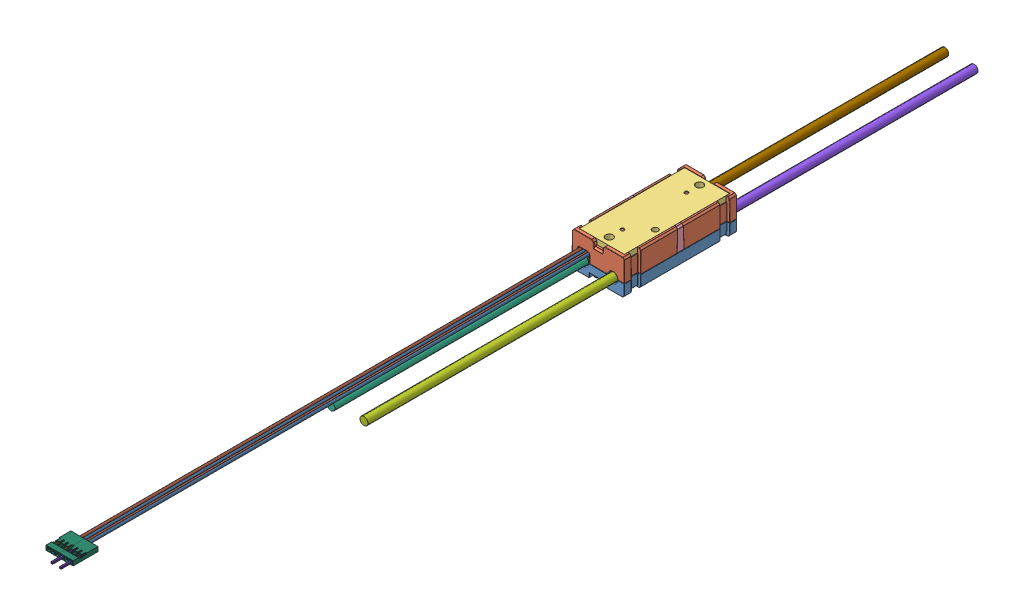
SolidWorks assembly Victor_SPX_217-9191, configuration Default. Lengths in mm.
Overall size (30.33 19.59 524.96).
27 component instances, 17 part files, 0 mates.
Components (placement in the parent):
- 217-9191-001 Rev3-1: 217-9191-001 Rev3 [Default] at origin size (29.5 7.19 63.51)
- 217-9191-002 Rev3-1: 217-9191-002 Rev3 [Default] at (0 2.7 0) size (29.5 14.96 63.52)
- 217-9191-003 Rev1-1: 217-9191-003 Rev1 [Default] at (0 9.35 0) size (25.3 3 59.3)
- 217-9191-004 Rev2-1: 217-9191-004 Rev2 [Default] at (6.795 4.495 0.0018) size (4.29 13.1 6.9)
- 217-9191-004 Rev2-2: 217-9191-004 Rev2 [Default] at (-6.795 4.495 0.0018) x (-1 0 0) z (0 0 -1) size (4.29 13.1 6.9)
- 217-9191-006 Rev2-1: 217-9191-006 Rev2 [Default] at (9.2964 8.362 8.8672) x (0 0 -1) z (1 0 0) size (6.08 10.55 6.08)
- 217-9191-911 Rev1_RED-1: 217-9191-911 Rev1_RED [Default] at (-8.25 0 21.5739) x (0.999994 0.00336 0) z (0 0 1) size (4.5 4.5 156.4)
- 217-9191-912 Rev1_Black-1: 217-9191-912 Rev1_Black [Default] at (8.25 0 19.558) x (0.697815 -0.716278 0) z (0 0 1) size (4.5 4.5 156.4)
- 217-9191-913 Rev1_White-1: 217-9191-913 Rev1_White [Default] at (8.25 0 -19.431) x (-0.549241 0.835664 0) z (0 0 -1) size (4.5 4.5 156.4)
- 217-9191-914 Rev1_Black-1: 217-9191-914 Rev1_Black [Default] at (-8.25 0 -19.431) x (-0.472775 0.881183 0) z (0 0 -1) size (4.5 4.5 156.4)
- 217-9191-915 Rev1-1: 217-9191-915 Rev1 [Default] at (-7.1946 -1.0626 7.493) x (0.370352 -0.928891 0) z (0 0 -1) size (6.7 1.5 308.78)
- 217-9191-916 Rev1-1: 217-9191-916 Rev1 [Default] at (-9.2392 -1.0626 7.493) x (-0.369925 -0.929062 0) z (0 0 -1) size (6.7 1.5 308.78)
- 217-9191-915 Rev1-2: 217-9191-915 Rev1 [Default] at (-6.3946 -1.0626 7.493) x (-0.103805 -0.994598 0) z (0 0 -1) size (6.7 1.5 308.78)
- 217-9191-916 Rev1-2: 217-9191-916 Rev1 [Default] at (-10.0392 -1.0626 7.493) x (0.104202 -0.994556 0) z (0 0 -1) size (6.7 1.5 308.78)
- 217-9191-005 Rev1-1: 217-9191-005 Rev1 [Default] at (-8.25 0 26.133) size (7.74 3.94 11.03)
- 217-9191-007 Rev1_92005A071-1: 217-9191-007 Rev1_92005A071 [Default] at (0 12.05 18) x (-0.856814 0 0.515625) z (0 -1 0) size (5 5 6.76)
- 217-9191-007 Rev1_92005A071-2: 217-9191-007 Rev1_92005A071 [Default] at (0 12.05 -18) x (1 0 0) z (0 -1 0) size (5 5 6.76)
- 217-9191-008 Rev1-1: 217-9191-008 Rev1 [Default] at (-78.6347 -3.05 22.1716) x (0.778462 0 -0.627691) z (0 -1 0) size (4.2 4.2 11.81)
- 217-9191-008 Rev1-2: 217-9191-008 Rev1 [Default] at (15.0561 -3.05 -46.2819) x (0.568576 0 0.822631) z (0 -1 0) size (4.2 4.2 11.81)
- 217-9191-008 Rev1-3: 217-9191-008 Rev1 [Default] at (-52.1 -3.05 -81.77) x (1 0 0) z (0 -1 0) size (4.2 4.2 11.81)
- 217-9191-008 Rev1-4: 217-9191-008 Rev1 [Default] at (-57.6 -3.05 -81.77) x (1 0 0) z (0 -1 0) size (4.2 4.2 11.81)
- 217-9090-018 Rev1-1: 217-9090-018 Rev1 [Default] at (-11.7479 3.8841 320.2778) size (7.66 2.5 14)
- 217-9090-019 Rev1-1: 217-9090-019 Rev1 [Default] at (-14.3254 4.0591 320.2778) size (1.6 1.6 12)
- 217-9090-019 Rev1-2: 217-9090-019 Rev1 [Default] at (-9.1704 4.0591 320.2778) size (1.6 1.6 12)
- 217-9090-018 Rev1-2: 217-9090-018 Rev1 [Default] at (-4.0879 3.8841 320.2778) size (7.66 2.5 14)
- 217-9191-017 Rev1-1: 217-9191-017 Rev1 [Default] at (-6.4904 3.8841 320.2778) size (1.6 1.6 28.85)
- 217-9191-017 Rev1-2: 217-9191-017 Rev1 [Default] at (-1.6854 3.8841 320.2778) size (1.6 1.6 28.85)
